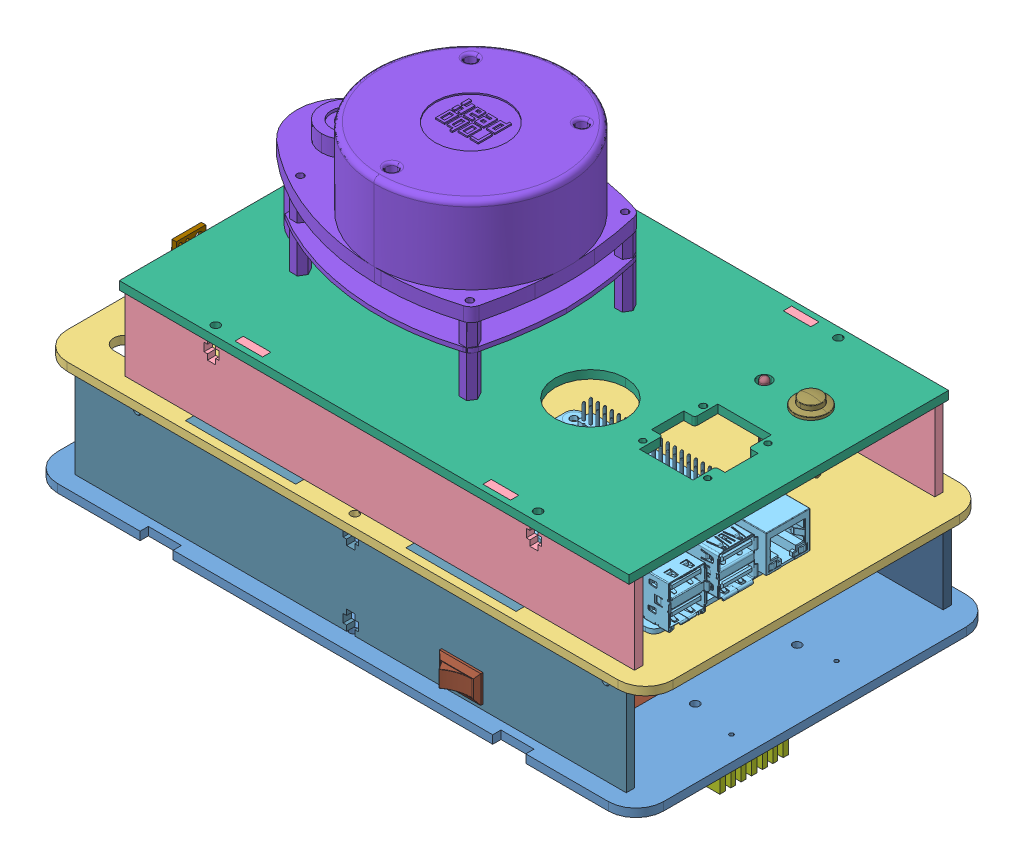
SolidWorks assembly 3, configuration Default. Lengths in mm.
Overall size (235.7 155.7 130).
26 component instances, 16 part files, 0 mates.
Components (placement in the parent):
- Assem_done(2)^3-1: Assem_done(2)^3 [Default] at origin size (235.7 155.7 130) (virtual)
  - Copy of basw1^Assem_done(2)_3-1: Copy of basw1^Assem_done(2)_3 [Default] at origin size (220 3 130) (virtual)
  - 18650 Cell Holder^Assem_done(2)_3-1: 18650 Cell Holder^Assem_done(2)_3 [Default] at (36.0932 3 0) x (1 0 0) z (0 1 0) size (78.6 83.7 21) (virtual)
  - base2^Assem_done(2)_3-1: base2^Assem_done(2)_3 [Default] at (0.47 37 0) size (220 3 124) (virtual)
  - winBase2^Assem_done(2)_3-1: winBase2^Assem_done(2)_3 [Default] at (25.47 51.5 -53) x (1 0 0) z (0 1 0) size (185 3 39) (virtual)
  - Raspberry Pi 4 Model B^Assem_done(2)_3-1: Raspberry Pi 4 Model B^Assem_done(2)_3 [Default] at (50.9427 40.8 13.9283) size (89 19.92 58.4) (virtual)
  - base3^Assem_done(2)_3-1: base3^Assem_done(2)_3 [Default] at (7.97 68 0) size (185 3 116) (virtual)
  - L298N_Stepper_motor_driver^Assem_done(2)_3-1: L298N_Stepper_motor_driver^Assem_done(2)_3 [Default] at (66.5 0 0) x (0 0 -1) z (-1 0 0) size (43 27 43) (virtual)
  - L298N_Stepper_motor_driver^Assem_done(2)_3-2: L298N_Stepper_motor_driver^Assem_done(2)_3 [Default] at (-66.5 0 0) x (0 0 1) z (1 0 0) size (43 27 43) (virtual)
  - rplidar_main_По умолчанию^Assem_done(2)_3-1: rplidar_main_По умолчанию^Assem_done(2)_3 [Default] at (-27.1712 95.6 1.9102) x (-0.99998 0 -0.006299) z (0.006299 0 -0.99998) size (98.5 57.7 70.02) (virtual)
  - winBase2^Assem_done(2)_3-2: winBase2^Assem_done(2)_3 [Default] at (25.47 51.5 56) x (1 0 0) z (0 1 0) size (185 3 39) (virtual)
  - TOF VL53L0X.stp^Assem_done(2)_3-1: TOF VL53L0X.stp^Assem_done(2)_3 [Default] at (-124.13 28.5484 -7.3714) x (0 0 -1) z (-1 0 0) size (10.7 14 2.7) (virtual)
  - winBase1^Assem_done(2)_3-1: winBase1^Assem_done(2)_3 [Default] at (0.47 20 -59) x (1 0 0) z (0 -1 0) size (200 3 40) (virtual)
  - Switch on off^Assem_done(2)_3-1: Switch on off^Assem_done(2)_3 [Default] at (40.9627 9.8337 51) x (0 1 0) z (1 0 0) size (10 19.96 15) (virtual)
  - Push_main_Défaut^Assem_done(2)_3-1: Push_main_Défaut^Assem_done(2)_3 [Default] at (80.7059 56 -27.817) size (12.02 24.8 12.02) (virtual)
  - Led_3mm_Verde_Transparente v1.step^Assem_done(2)_3-1: Led_3mm_Verde_Transparente v1.step^Assem_done(2)_3 [Default] at (63.7826 67 -27.817) x (-0.420564 0 0.907263) z (0 1 0) size (3.58 3.85 31.6) (virtual)
  - winBase1_LEFT^Assem_done(2)_3-1: winBase1_LEFT^Assem_done(2)_3 [Default] at (0.47 20 56) x (1 0 0) z (0 -1 0) size (200 3 40) (virtual)
  - LM2596^Assem_done(2)_3-1: LM2596^Assem_done(2)_3 [Default] at (14.0389 -5 0) x (0 0 -1) z (-1 0 0) size (43.2 15.15 21.25) (virtual)
  - hexagonal_spacer_FF_M3_H05_HEX5_pass_through.step^Assem_done(2)_3-1: hexagonal_spacer_FF_M3_H05_HEX5_pass_through.step^Assem_done(2)_3 [Default] at (-8.6383 -5 20) x (1 0 0) z (0 1 0) size (5.78 5.01 5.38) (virtual)
  - hexagonal_spacer_FF_M3_H05_HEX5_pass_through.step^Assem_done(2)_3-2: hexagonal_spacer_FF_M3_H05_HEX5_pass_through.step^Assem_done(2)_3 [Default] at (5.9139 -5 -15.1) x (1 0 0) z (0 1 0) size (5.78 5.01 5.38) (virtual)
  - hexagonal_spacer_FF_M3_H05_HEX5_pass_through.step^Assem_done(2)_3-3: hexagonal_spacer_FF_M3_H05_HEX5_pass_through.step^Assem_done(2)_3 [Default] at (22.1639 -5 15.1) x (1 0 0) z (0 1 0) size (5.78 5.01 5.38) (virtual)
  - hexagonal_spacer_FF_M3_H05_HEX5_pass_through.step^Assem_done(2)_3-4: hexagonal_spacer_FF_M3_H05_HEX5_pass_through.step^Assem_done(2)_3 [Default] at (-27.6383 -5 -20) x (1 0 0) z (0 1 0) size (5.78 5.01 5.38) (virtual)
  - hexagonal_spacer_FF_M3_H05_HEX5_pass_through.step^Assem_done(2)_3-5: hexagonal_spacer_FF_M3_H05_HEX5_pass_through.step^Assem_done(2)_3 [Default] at (-95.2117 40 -29.5113) x (1 0 0) z (0 1 0) size (5.78 5.01 5.38) (virtual)
  - hexagonal_spacer_FF_M3_H05_HEX5_pass_through.step^Assem_done(2)_3-6: hexagonal_spacer_FF_M3_H05_HEX5_pass_through.step^Assem_done(2)_3 [Default] at (-6.1116 40 -29.401) x (0.959244 0 0.282579) z (0 1 0) size (5.78 5.01 5.38) (virtual)
  - hexagonal_spacer_FF_M3_H05_HEX5_pass_through.step^Assem_done(2)_3-7: hexagonal_spacer_FF_M3_H05_HEX5_pass_through.step^Assem_done(2)_3 [Default] at (-94.9555 40 29.5285) x (1 0 0) z (0 1 0) size (5.78 5.01 5.38) (virtual)
  - hexagonal_spacer_FF_M3_H05_HEX5_pass_through.step^Assem_done(2)_3-8: hexagonal_spacer_FF_M3_H05_HEX5_pass_through.step^Assem_done(2)_3 [Default] at (-6.1057 40 29.029) x (1 0 0) z (0 1 0) size (5.78 5.01 5.38) (virtual)
